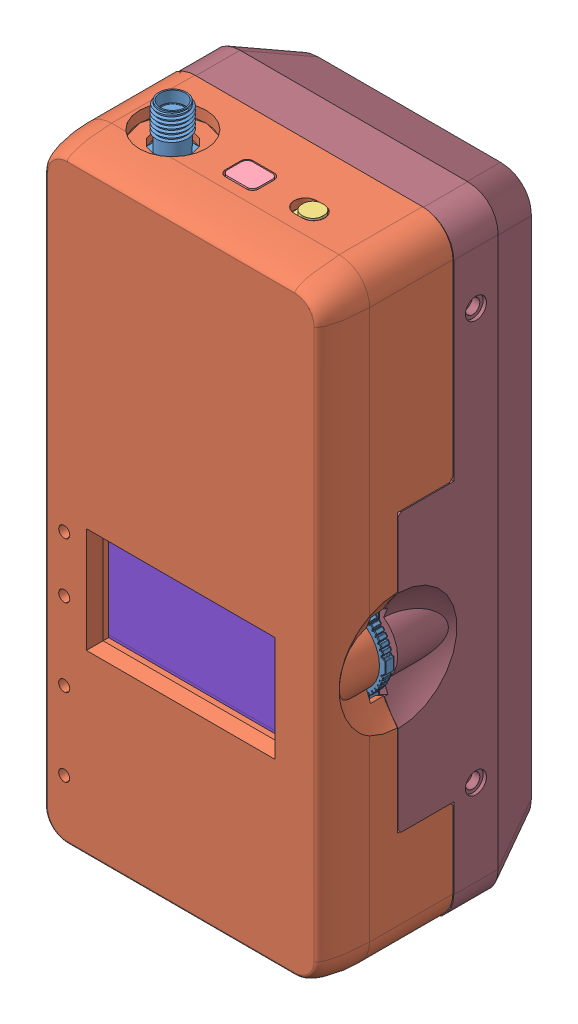
SolidWorks assembly MTL-2, configuration Default. Lengths in mm.
Overall size (53.19 114.66 41.12).
26 component instances, 13 part files, 2 mates.
Components (placement in the parent):
- MTL_02-01a.step-1: MTL_02-01a.step [По умолчанию] at (15.0166 10.5569 84.5103) size (48.17 109.55 13.53)
- Middle-1: Middle [По умолчанию] at (36.0298 60.5518 84.5103) x (1 -0.00028 0) z (0 0 1) size (52.9 110.2 32.1)
- SW1-1: SW1 [По умолчанию] at (47.3923 115.7706 85.1043) x (-0.999962 0.000076 0.008726) z (0 -0.999962 0.008727) size (7 6 5)
- SW1-2: SW1 [По умолчанию] at (9.6836 37.2786 85.0832) x (0.000076 -0.999848 0.017452) z (0.999962 -0.000076 -0.008726) size (7 6 5)
- BT1-L-1: BT1-L [По умолчанию] at (36.0015 115.5484 85.0548) x (1 0 0) z (0 -0.999962 0.008727) size (8.5 6.5 4)
- OLED-SSD1306-128x64-i2c-1: OLED-SSD1306-128x64-i2c [По умолчанию] at (18.301 30.2339 91.2322) size (35.4 33.8 11.5)
  - OLED-SSD1306-128x64-i2c.step-1: OLED-SSD1306-128x64-i2c.step [По умолчанию] at origin size (35.4 33.8 11.5)
    - ____________________ __________.step-1: ____________________ __________.step [По умолчанию] at origin size (10.16 2.54 11.2)
      - Body001.step-1: Body001.step [По умолчанию] at (13.9 32.33 0) size (2.54 2.54 11.2)
      - Body001.step-2: Body001.step [По умолчанию] at (16.44 32.33 0) size (2.54 2.54 11.2)
      - Body001.step-3: Body001.step [По умолчанию] at (18.98 32.33 0) size (2.54 2.54 11.2)
      - Body001.step-4: Body001.step [По умолчанию] at (21.52 32.33 0) size (2.54 2.54 11.2)
    - ________________ __________.step-1: ________________ __________.step [По умолчанию] at origin size (35.4 33.8 1.25)
    - __________ ______________.step-1: __________ ______________.step [По умолчанию] at (17.6 3.5 1.6) size (22 10.7 3.4)
    - ______________.step-1: ______________.step [По умолчанию] at origin size (34.5 23 2)
    - ______________-0.step-1: ______________-0.step [По умолчанию] at origin size (15 5 0.16)
- BC-18650-PC4-2: BC-18650-PC4 [По умолчанию] at (36.0135 64.8265 82.3064) x (1 0 0) z (0 1 0) size (40.5 24.7 78)
  - User Library-BC-18650-PC4.STEP-1: User Library-BC-18650-PC4.STEP [По умолчанию] at origin size (40.5 24.7 78)
    - BC-18650-PC4.STEP.STEP-1: BC-18650-PC4.STEP.STEP [По умолчанию] at origin size (40.5 24.7 78)
      - ____________2^__________ ____________________________ BC-18650-PC4_____ __________________.STEP.STEP-1: ____________2^__________ ____________________________ BC-18650-PC4_____ __________________.STEP.STEP [По умолчанию] x (1 0 0) z (0 1 0) size (40.5 78 21.5)
      - ____________3^__________ ____________________________ BC-18650-PC4_____ __________________.STEP.STEP-1: ____________3^__________ ____________________________ BC-18650-PC4_____ __________________.STEP.STEP [По умолчанию] at (-9.65 0 0) x (0 0 1) z (-1 0 0) size (5.89 19.7 6.6)
      - ____________3^__________ ____________________________ BC-18650-PC4_____ __________________.STEP.STEP-2: ____________3^__________ ____________________________ BC-18650-PC4_____ __________________.STEP.STEP [По умолчанию] at (-9.65 0 0) x (0 0 -1) z (1 0 0) size (5.89 19.7 6.6)
      - ____________3^__________ ____________________________ BC-18650-PC4_____ __________________.STEP.STEP-3: ____________3^__________ ____________________________ BC-18650-PC4_____ __________________.STEP.STEP [По умолчанию] at (9.65 0 0) x (0 0 1) z (-1 0 0) size (5.89 19.7 6.6)
      - ____________3^__________ ____________________________ BC-18650-PC4_____ __________________.STEP.STEP-4: ____________3^__________ ____________________________ BC-18650-PC4_____ __________________.STEP.STEP [По умолчанию] at (9.65 0 0) x (0 0 -1) z (1 0 0) size (5.89 19.7 6.6)
- VK2828U7-1: VK2828U7 [По умолчанию] at (40.0977 83.5972 92.3389) x (0.999924 -0.008726 -0.008727) z (-0.008726 0.000076 -0.999962) size (28.5 28.5 8.4)
- Back-1: Back [По умолчанию] at (36.1721 60.4947 60.4927) size (52 110 28.11)
Mates (geometry in assembly coordinates):
- Концентричный1: concentric anti-aligned: circle of MTL_02-01a.step-1; circle of Midle-1
- Совпадение2: coincident anti-aligned: plane of MTL_02-01a.step-1 through (36.6303 60.8557 84.5103) normal (0 0 1); plane of Midle-1 through (36.0298 60.5518 84.5103) normal (0 0 -1)
